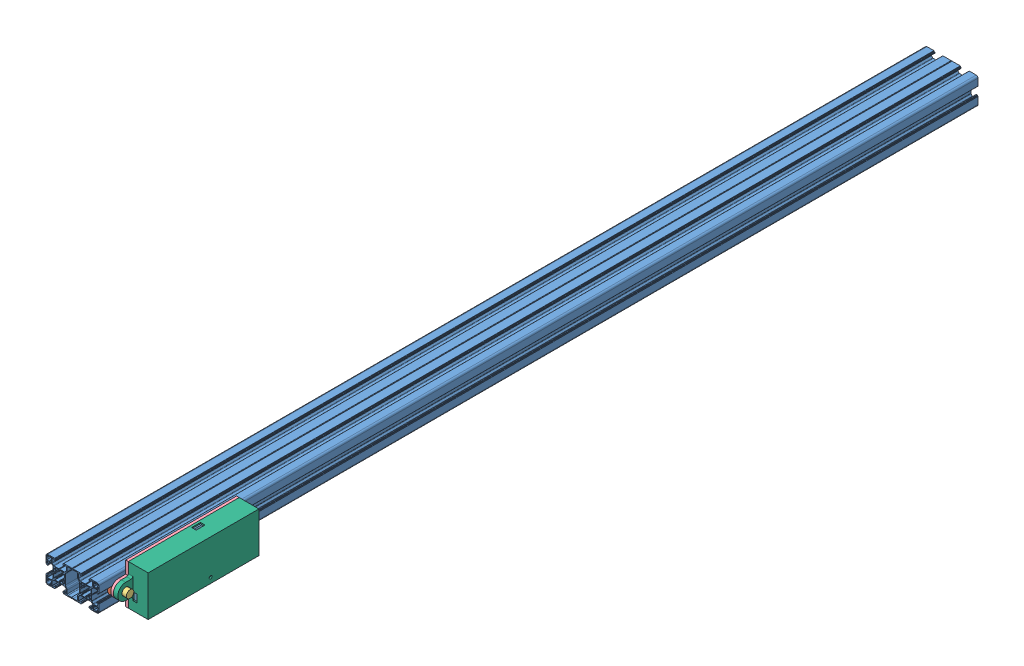
SolidWorks assembly Угломер направляющей, configuration Default. Lengths in mm.
Overall size (85.5 50.19 1000).
16 component instances, 11 part files, 31 mates.
Components (placement in the parent):
- Конструкционный профиль направляющей 30на60SLX-1: Конструкционный профиль направляющей 30на60SLX [00] at (268.0525 -771.9763 1080.4966) size (60 30 1000)
- сухарь (гайка т-образная)-1: сухарь (гайка т-образная) [По умолчанию] at (306.3525 -772.4132 908.9268) x (0 -1 0) z (0 0 1) size (15 5.5 13)
- винт м5 с цилиндрической головкой и шестигранным отверстием-1: винт м5 с цилиндрической головкой и шестигранным отверстием [По умолчанию] at (321.0525 -771.9414 915.786) x (0 -0.998395 0.056628) z (1 0 0) size (8.5 8.5 21)
- корпус_платы-1: корпус_платы [По умолчанию] at (313.0525 -750.4414 925.326) x (0 0 1) z (1 0 0) size (160.08 46 5.5)
- плата-1: плата [По умолчанию] at (318.5525 -791.9414 926.826) x (0 0 1) z (-1 0 0) size (120 40 1.5)
- крышка корпуса платы-1: крышка корпуса платы [По умолчанию] at (337.0525 -793.4414 1048.326) x (0 0 -1) z (1 0 0) size (160.08 46 22.5)
- сухарь (гайка т-образная)-2: сухарь (гайка т-образная) [По умолчанию] at (306.3525 -772.4132 1051.0068) x (0 -1 0) z (0 0 1) size (15 5.5 13)
- винт м5 с цилиндрической головкой и шестигранным отверстием-3: винт м5 с цилиндрической головкой и шестигранным отверстием [По умолчанию] at (321.0525 -771.9414 1057.866) x (0 0.587872 0.808954) z (1 0 0) size (8.5 8.5 21)
- Сборка1^Угломер направляющей-1: Сборка1^Угломер направляющей [По умолчанию] at origin (virtual)
- Переключатель SPST - KCD1-11 (ON-OFF).step-1: Переключатель SPST - KCD1-11 (ON-OFF).step [По умолчанию] at (328.7141 -794.9414 992.176) x (0 0 -1) z (0 -1 0) size (15 10.5 19.39)
- ArduinoNano-USB-mini.step-1: ArduinoNano-USB-mini.step [По умолчанию] at (317.4125 -799.2749 1047.0661) x (0 0 -1) z (1 0 0) size (44.46 17.85 7.11)
- АКБ 2S 800 mAh-1: АКБ 2S 800 mAh [По умолчанию] at (327.7525 -772.216 950.956) x (0 0 1) z (0 1 0) size (39 25.55 36.3)
  - АКБ-1: АКБ [По умолчанию] at (0 0 8.95) size (34.12 24.7 16.7) (hidden)
  - АКБ-2: АКБ [По умолчанию] at (0 0 -8.95) size (34.12 24.7 16.7) (hidden)
  - Корпус АКБ-1: Корпус АКБ [По умолчанию] at origin size (38 18.4 36.3)
  - Крышка корпуса-1: Крышка корпуса [По умолчанию] at (-18.5 0 0) x (0 0 -1) z (1 0 0) size (36.3 18.4 2.5)
Mates (geometry in assembly coordinates):
- Совпадение4: coincident anti-aligned: plane of Конструкционный профиль направляющей 30на60SLX-1 through (310.8525 -767.8763 80.4966) normal (-1 0 0); plane of сухарь (гайка т-образная)-1 through (310.8525 -764.5763 921.9268) normal (1 0 0)
- Параллельность1: parallel aligned: plane of Конструкционный профиль направляющей 30на60SLX-1 through (313.0525 -756.9763 80.4966) normal (1 0 0); plane of сухарь (гайка т-образная)-1 through (311.8525 -768.0763 921.9268) normal (1 0 0)
- Совпадение6: coincident anti-aligned: plane of Конструкционный профиль направляющей 30на60SLX-1 through (313.0525 -776.0763 80.4966) normal (0 1 0); plane of сухарь (гайка т-образная)-1 through (311.8525 -776.0763 921.9268) normal (0 -1 0)
- Концентричный3: concentric aligned: cylinder of сухарь (гайка т-образная)-1 through (311.8525 -771.9414 915.786) axis (1 0 0) radius 2.75; cylinder of винт м5 с цилиндрической головкой и шестигранным отверстием-1 through (305.0525 -771.9414 915.786) axis (1 0 0) radius 2.5
- Совпадение7: coincident anti-aligned: plane of Конструкционный профиль направляющей 30на60SLX-1 through (313.0525 -756.9763 80.4966) normal (1 0 0); plane of корпус_платы-1 through (313.0525 -750.4414 925.326) normal (-1 0 0)
- Параллельность2: parallel aligned: plane of корпус_платы-1 through (316.0525 -750.4414 925.326) normal (1 0 0); plane of плата-1 through (318.5525 -791.9414 926.826) normal (1 0 0)
- Параллельность3: parallel aligned: plane of Конструкционный профиль направляющей 30на60SLX-1 through (313.0525 -786.9763 80.4966) normal (0 -1 0); plane of плата-1 through (317.0525 -791.9414 926.826) normal (0 -1 0)
- Концентричный6: concentric aligned: circle of корпус_платы-1; circle of плата-1
- Совпадение12: coincident aligned: plane of корпус_платы-1 through (318.5525 -789.9414 928.826) normal (1 0 0); plane of плата-1 through (318.5525 -791.9414 926.826) normal (1 0 0)
- Концентричный8: concentric anti-aligned: cylinder of винт м5 с цилиндрической головкой и шестигранным отверстием-1 through (305.0525 -771.9414 915.786) axis (1 0 0) radius 2.5; cylinder of корпус_платы-1 through (340.8389 -771.9414 915.786) axis (-1 0 0) radius 3.5
- Концентричный9: concentric aligned: circle of корпус_платы-1; cylinder of крышка корпуса платы-1 through (321.0525 -771.9414 1057.866) axis (-1 0 0) radius 3.5
- Концентричный10: concentric aligned: circle of корпус_платы-1; circle of крышка корпуса платы-1
- Совпадение20: coincident anti-aligned: plane of Конструкционный профиль направляющей 30на60SLX-1 through (310.8525 -776.0763 80.4966) normal (-1 0 0); plane of сухарь (гайка т-образная)-2 through (310.8525 -776.0763 1064.0068) normal (1 0 0)
- Концентричный15: concentric aligned: circle of корпус_платы-1; circle of сухарь (гайка т-образная)-2
- Концентричный16: concentric aligned: circle of крышка корпуса платы-1; cylinder of винт м5 с цилиндрической головкой и шестигранным отверстием-3 through (305.0525 -771.9414 1057.866) axis (1 0 0) radius 2.5
- Параллельность8: parallel aligned: plane of плата-1 through (318.5525 -791.9414 926.826) normal (1 0 0); plane of ArduinoNano-USB-mini.step-1 through (321.5525 -780.1164 1020.346) normal (1 0 0)
- Совпадение27: coincident anti-aligned: plane of плата-1 through (318.5525 -791.9414 926.826) normal (1 0 0); plane of ArduinoNano-USB-mini.step-1 through (318.5525 -774.9064 1039.421) normal (-1 0 0)
- Параллельность11: parallel aligned: plane of плата-1 through (317.0525 -791.9414 926.826) normal (0 -1 0); plane of ArduinoNano-USB-mini.step-1 through (320.0525 -789.0414 1041.971) normal (0 -1 0)
- Концентричный17: concentric aligned: cylinder of корпус_платы-1 through (318.5525 -753.9414 928.826) axis (-1 0 0) radius 1; circle of плата-1
- Расстояние1: distance = 4 mm: plane of assembly; line of assembly; plane of плата-1 through (317.0525 -791.9414 926.826) normal (0 -1 0)
- Расстояние2: distance = 8.7 mm: plane of assembly; line of assembly; plane of плата-1 through (317.0525 -791.9414 1046.826) normal (0 0 1)
- Расстояние5: distance = 7.13 mm aligned: plane of плата-1 through (317.0525 -791.9414 926.826) normal (0 0 -1); plane of АКБ 2S 800 mAh-1/АКБ-2 through (327.7525 -781.166 933.956) normal (0 0 -1)
- Совпадение36: coincident anti-aligned: plane of крышка корпуса платы-1 through (321.0525 -771.9414 1057.866) normal (1 0 0); plane of винт м5 с цилиндрической головкой и шестигранным отверстием-3 through (321.0525 -771.9414 1057.866) normal (-1 0 0)
- Параллельность16: parallel aligned: plane of Конструкционный профиль направляющей 30на60SLX-1 through (268.0525 -771.9763 1080.4966) normal (0 0 1); plane of сухарь (гайка т-образная)-2 through (306.3525 -772.4132 1064.0068) normal (0 0 1)
- Совпадение38: coincident anti-aligned: plane of винт м5 с цилиндрической головкой и шестигранным отверстием-1 through (321.0525 -771.9414 915.786) normal (-1 0 0); plane of крышка корпуса платы-1 through (321.0525 -771.9414 915.786) normal (1 0 0)
- Заблокировать1: lock: unknown of Конструкционный профиль направляющей 30на60SLX-1; unknown of корпус_платы-1
- Совпадение40: coincident anti-aligned: plane of крышка корпуса платы-1 through (338.5525 -794.9414 923.826) normal (0 -1 0); plane of Переключатель SPST - KCD1-11 (ON-OFF).step-1 through (328.7141 -794.9414 992.176) normal (0 1 0)
- Совпадение41: coincident anti-aligned: plane of крышка корпуса платы-1 through (333.5525 -784.9414 985.326) normal (0 0 1); plane of Переключатель SPST - KCD1-11 (ON-OFF).step-1 through (332.8641 -793.8174 985.326) normal (0 0 -1)
- Заблокировать2: lock: unknown of крышка корпуса платы-1; unknown of Переключатель SPST - KCD1-11 (ON-OFF).step-1
- Совпадение42: coincident anti-aligned: plane of плата-1 through (318.5525 -791.9414 926.826) normal (1 0 0); plane of АКБ 2S 800 mAh-1/Корпус АКБ-1 through (318.5525 -785.166 969.456) normal (-1 0 0)
- Совпадение43: coincident anti-aligned: plane of корпус_платы-1 through (316.0525 -750.4414 925.326) normal (1 0 0); plane of крышка корпуса платы-1 through (316.0525 -793.4414 1048.326) normal (-1 0 0)
